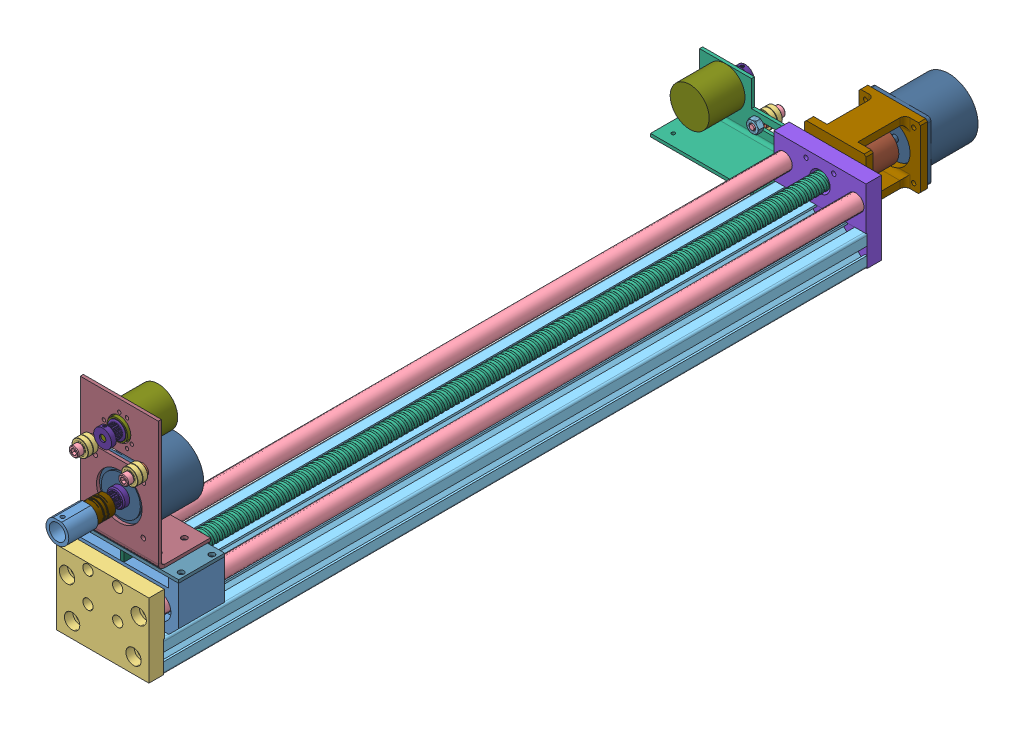
SolidWorks assembly BallScrewAssm2Motors, configuration Default. Lengths in mm.
Overall size (227 210 870.18).
53 component instances, 24 part files, 41 mates.
Components (placement in the parent):
- BallScrewBlock-1: BallScrewBlock [Default] at (0 32 293.5303) size (110 48 45)
- BallScrewCap-1: BallScrewCap [Default] at (0 51.5 283.5303) size (48.01 39 10)
- BallScrewEnd-1: BallScrewEnd [Default] at (0 36 357.5) x (-1 0 0) z (0 0 -1) size (90 72 15)
- BallScrewGuide-1: BallScrewGuide [Default] at (35 51.5 347.5) x (-0.923728 -0.383049 0) z (0.383049 -0.923728 0) size (16 705 16)
- Extrusion Base-1: Extrusion Base [Default] at origin size (90 30 687)
- BallScrewGuide-2: BallScrewGuide [Default] at (-35 51.5 347.5) x (-0.928239 -0.371985 0) z (0.371985 -0.928239 0) size (16 705 16)
- BallScrew-1: BallScrew [Default] at (0 51.5 347.5) x (-0.999726 0.023415 0) z (-0.023415 -0.999726 0) size (16.82 726.5 16)
- BallScrewBearing-1: BallScrewBearing [Default] at (0 51.5 342.5) x (1 0 0) z (0 -1 0) size (27 5 27)
- BallScrewMotorEnd-1: BallScrewMotorEnd [Default] at (0 36 -357.5) size (90 72 15)
- MotorMount-1: MotorMount [Default] at (0 51.5 -387.5) x (0 1 0) z (0 0 1) size (60 60 60)
- Motor-1: Motor [Default] at (0 51.5 -417.5) x (0 1 0) z (0 0 1) size (57.15 57.15 71.37)
- MotorBallCoupler-1: MotorBallCoupler [Default] at (0 51.5 -404.5) x (-0.999726 0.023415 0) z (0 0 1) size (30 30 34)
- CutPulley-1: CutPulley [Default] at (0 51.5 -404.5) x (0.023415 0.999726 0) z (-0.999726 0.023415 0) size (12.94 6.35 12.94)
- RodMotorAssm-1: RodMotorAssm [Default] at (0 86 316.0303) x (-1 0 0) z (0 0 -1) size (110 139 114.25)
  - HorizontalMotorMount-2: HorizontalMotorMount [Default] at origin size (76.2 127 50.8)
  - Motor-1: Motor [Default] at (0 41.45 -22.4) x (-1 0 0) z (0 0 -1) size (57.15 57.15 71.37)
  - MotorSupport-1: MotorSupport [Default] at (0 -6 0) size (110 3 45)
  - MotorPlatformSupport-1: MotorPlatformSupport [Default] at (0 -15 0) x (0 0 -1) z (1 0 0) size (45 12 3)
  - Encoder-1: Encoder [Default] at (0 98.6 12.6) x (-1 0 0) z (0 0 -1) size (38 38 53)
  - 1375K39_MXL Series Timing Belt Pulley-1: 1375K39_MXL Series Timing Belt Pulley [1375K39] at (0 41.45 -31.0741) x (0 0 -1) z (0.414927 -0.909855 0) size (14.3 17.4 17.4)
  - 6208K433_Clamping Precision Flexible Shaft Coupling-1: 6208K433_Clamping Precision Flexible Shaft Coupling [6208K433] at (0 41.45 -47.7492) size (20.03 19.05 19.05)
  - 1375K39_MXL Series Timing Belt Pulley-2: 1375K39_MXL Series Timing Belt Pulley [1375K39] at (0 98.6 -34.5501) x (0 0 1) z (0.089879 0.995953 0) size (14.3 17.4 17.4)
  - MotorRodCoupler-1: MotorRodCoupler [Default] at (0 41.45 -85.8492) x (-1 0 0) z (0 0 -1) size (22.23 21.43 38.1)
  - Idler-1: Idler [Default] at (25.4 75.7798 -30.4193) x (-0.670496 -0.741913 0) z (0 0 -1) size (15.88 15.88 29.4)
    - IdlerSpacer-1: IdlerSpacer [Default] at (0 0 -5.0193) x (1 0 0) z (0 -1 0) size (10.79 3 10.79)
    - 60355K701_Ball Bearing-1: 60355K701_Ball Bearing [60355K701] at (0 0 0.4699) size (15.88 15.88 4.98)
    - 91251A541_Black-Oxide Alloy Steel Socket Head Screw-1: 91251A541_Black-Oxide Alloy Steel Socket Head Screw [91251A541] at origin size (9.53 9.53 29.4)
    - 60355K701_Ball Bearing-2: 60355K701_Ball Bearing [60355K701] at (0 0 5.4483) size (15.88 15.88 4.98)
    - 95462A029_Medium-Strength Steel Hex Nut-1: 95462A029_Medium-Strength Steel Hex Nut [95462A029] at (0 0 -10.7974) size (11.11 12.83 6.51)
  - Idler-2: Idler [Default] at (-22.9813 75.7798 -30.4193) x (-0.670496 -0.741913 0) z (0 0 -1) size (15.88 15.88 29.4)
    - IdlerSpacer-1: IdlerSpacer [Default] at (0 0 -5.0193) x (1 0 0) z (0 -1 0) size (10.79 3 10.79)
    - 60355K701_Ball Bearing-1: 60355K701_Ball Bearing [60355K701] at (0 0 0.4699) size (15.88 15.88 4.98)
    - 91251A541_Black-Oxide Alloy Steel Socket Head Screw-1: 91251A541_Black-Oxide Alloy Steel Socket Head Screw [91251A541] at origin size (9.53 9.53 29.4)
    - 60355K701_Ball Bearing-2: 60355K701_Ball Bearing [60355K701] at (0 0 5.4483) size (15.88 15.88 4.98)
    - 95462A029_Medium-Strength Steel Hex Nut-1: 95462A029_Medium-Strength Steel Hex Nut [95462A029] at (0 0 -10.7974) size (11.11 12.83 6.51)
- BallEncoderAssm-1: BallEncoderAssm [Default] at (-45 3 -399.9402) x (-1 0 0) z (0 0 -1) size (131.66 50.8 70.38)
  - Encoder-1: Encoder [Default] at (101.6 28.75 -38) size (38 38 53)
  - BallEncoderHolder-1: BallEncoderHolder [Default] at origin size (127 50.8 50.8)
  - 1375K39_MXL Series Timing Belt Pulley-1: 1375K39_MXL Series Timing Belt Pulley [1375K39] at (101.6 28.75 9.1501) x (0 0 -1) z (1 0 0) size (14.3 17.4 17.4)
  - Idler-1: Idler [Default] at (6.35 12.875 5.0193) x (-0.556818 0.830635 0) z (0 0 1) size (15.88 15.88 29.4)
    - IdlerSpacer-1: IdlerSpacer [Default] at (0 0 -5.0193) x (1 0 0) z (0 -1 0) size (10.79 3 10.79)
    - 60355K701_Ball Bearing-1: 60355K701_Ball Bearing [60355K701] at (0 0 0.4699) size (15.88 15.88 4.98)
    - 91251A541_Black-Oxide Alloy Steel Socket Head Screw-1: 91251A541_Black-Oxide Alloy Steel Socket Head Screw [91251A541] at origin size (9.53 9.53 29.4)
    - 60355K701_Ball Bearing-2: 60355K701_Ball Bearing [60355K701] at (0 0 5.4483) size (15.88 15.88 4.98)
    - 95462A029_Medium-Strength Steel Hex Nut-1: 95462A029_Medium-Strength Steel Hex Nut [95462A029] at (0 0 -10.7974) size (11.11 12.83 6.51)
  - Idler-2: Idler [Default] at (69.85 12.875 5.0193) x (-0.099236 -0.995064 0) z (0 0 1) size (15.88 15.88 29.4)
    - IdlerSpacer-1: IdlerSpacer [Default] at (0 0 -5.0193) x (1 0 0) z (0 -1 0) size (10.79 3 10.79)
    - 60355K701_Ball Bearing-1: 60355K701_Ball Bearing [60355K701] at (0 0 0.4699) size (15.88 15.88 4.98)
    - 91251A541_Black-Oxide Alloy Steel Socket Head Screw-1: 91251A541_Black-Oxide Alloy Steel Socket Head Screw [91251A541] at origin size (9.53 9.53 29.4)
    - 60355K701_Ball Bearing-2: 60355K701_Ball Bearing [60355K701] at (0 0 5.4483) size (15.88 15.88 4.98)
    - 95462A029_Medium-Strength Steel Hex Nut-1: 95462A029_Medium-Strength Steel Hex Nut [95462A029] at (0 0 -10.7974) size (11.11 12.83 6.51)
  - 95462A029_Medium-Strength Steel Hex Nut-1: 95462A029_Medium-Strength Steel Hex Nut [95462A029] at (6.35 12.875 -5.7781) x (-0.99776 -0.066901 0) z (0 0 1) size (11.11 12.83 6.51)
  - 95462A029_Medium-Strength Steel Hex Nut-2: 95462A029_Medium-Strength Steel Hex Nut [95462A029] at (69.85 12.875 -5.7781) x (0.911368 0.411591 0) z (0 0 1) size (11.11 12.83 6.51)
Mates (geometry in assembly coordinates):
- Coincident1: coordinate: point of Extrusion Base-1
- Coincident2: coincident anti-aligned: plane of BallScrewEnd-1 through (0 36 343.5) normal (0 0 -1); plane of Extrusion Base-1 through (0 0 343.5) normal (0 0 1)
- Concentric1: concentric aligned: cylinder of BallScrewEnd-1 through (30 15 357.5) axis (0 0 1) radius 4.5; cylinder of Extrusion Base-1 through (30 15 343.5) axis (0 0 1) radius 3.5
- Concentric2: concentric aligned: cylinder of BallScrewEnd-1 through (-30 15 357.5) axis (0 0 1) radius 4.5; cylinder of Extrusion Base-1 through (-30 15 343.5) axis (0 0 1) radius 3.5
- Concentric3: concentric aligned: cylinder of BallScrewEnd-1 through (35 51.5 357.5) axis (0 0 1) radius 4.5; cylinder of BallScrewGuide-1 through (35 51.5 347.5) axis (0 0 1) radius 3.5
- Coincident3: coincident aligned: plane of BallScrewEnd-1 through (35 51.5 347.5) normal (0 0 -1); circle of BallScrewGuide-1
- Concentric4: concentric aligned: cylinder of BallScrewBlock-1 through (35 51.5 293.5303) axis (0 0 1) radius 8; cylinder of BallScrewGuide-1 through (35 51.5 -357.5) axis (0 0 1) radius 8
- Concentric5: concentric anti-aligned: cylinder of BallScrewBlock-1 through (0 51.5 293.5303) axis (0 0 1) radius 8; cylinder of BallScrewCap-1 through (0 51.5 293.5303) axis (0 0 -1) radius 8
- Coincident4: coincident: plane of BallScrewBlock-1 through (0 32 293.5303) normal (0 0 -1); line of BallScrewCap-1 through (14 71 293.5303) axis (-1 0 0)
- Concentric6: concentric anti-aligned: cylinder of BallScrewBlock-1 through (-13.435 64.935 293.5303) axis (0 0 -1) radius 2.5; cylinder of BallScrewCap-1 through (-13.435 64.935 293.5303) axis (0 0 1) radius 3.3
- Concentric7: concentric anti-aligned: cylinder of BallScrewEnd-1 through (-35 51.5 347.5) axis (0 0 -1) radius 8; cylinder of BallScrewGuide-2 through (-35 51.5 -357.5) axis (0 0 1) radius 8
- Coincident5: coincident aligned: plane of BallScrewEnd-1 through (-35 51.5 347.5) normal (0 0 -1); circle of BallScrewGuide-2
- Concentric8: concentric aligned: cylinder of BallScrewBlock-1 through (-35 51.5 293.5303) axis (0 0 1) radius 8; cylinder of BallScrewGuide-2 through (-35 51.5 -357.5) axis (0 0 1) radius 8
- Concentric9: concentric anti-aligned: cylinder of BallScrewEnd-1 through (0 51.5 347.5) axis (0 0 -1) radius 13.5; cylinder of BallScrew-1 through (0 51.5 342.5) axis (0 0 1) radius 7.25
- Coincident6: coincident anti-aligned: plane of BallScrewEnd-1 through (0 51.5 347.5) normal (0 0 -1); plane of BallScrew-1 through (0 51.5 347.5) normal (0 0 1)
- Concentric10: concentric anti-aligned: cylinder of BallScrew-1 through (0 51.5 342.5) axis (0 0 1) radius 7.25; cylinder of BallScrewBearing-1 through (0 51.5 347.5) axis (0 0 -1) radius 7.5
- Coincident7: coincident anti-aligned: plane of BallScrewEnd-1 through (0 51.5 347.5) normal (0 0 -1); circle of BallScrewBearing-1
- Concentric11: concentric aligned: cylinder of BallScrewGuide-1 through (35 51.5 -357.5) axis (0 0 1) radius 8; cylinder of BallScrewMotorEnd-1 through (35 51.5 -357.5) axis (0 0 1) radius 8
- Concentric12: concentric aligned: cylinder of BallScrewGuide-2 through (-35 51.5 -357.5) axis (0 0 1) radius 8; cylinder of BallScrewMotorEnd-1 through (-35 51.5 -357.5) axis (0 0 1) radius 8
- Coincident8: coincident anti-aligned: plane of Extrusion Base-1 through (0 0 -343.5) normal (0 0 -1); plane of BallScrewMotorEnd-1 through (0 36 -343.5) normal (0 0 1)
- Concentric13: concentric anti-aligned: cylinder of MotorMount-1 through (-13.5 38 -357.5) axis (0 0 1) radius 2.75; cylinder of BallScrewMotorEnd-1 through (-13.5 38 -357.5) axis (0 0 -1) radius 2.1
- Concentric14: concentric anti-aligned: cylinder of MotorMount-1 through (-13.5 65 -357.5) axis (0 0 1) radius 2.75; cylinder of BallScrewMotorEnd-1 through (-13.5 65 -357.5) axis (0 0 -1) radius 2.1
- Coincident9: coincident anti-aligned: plane of BallScrewMotorEnd-1 through (0 36 -357.5) normal (0 0 -1); plane of MotorMount-1 through (30 81.5 -357.5) normal (0 0 1)
- Concentric15: concentric aligned: cylinder of MotorMount-1 through (0 51.5 -417.5) axis (0 0 1) radius 20; cylinder of Motor-1 through (0 51.5 -468.3) axis (0 0 1) radius 28.575
- Concentric16: concentric anti-aligned: circle of MotorMount-1; circle of Motor-1
- Coincident10: coincident: plane of MotorMount-1 through (30 81.5 -417.5) normal (0 0 -1); line of Motor-1 through (-28.575 76.9 -417.5) axis (0 -1 0)
- Concentric17: concentric anti-aligned: cylinder of Motor-1 through (0 51.5 -396.926) axis (0 0 -1) radius 3.175; cylinder of MotorBallCoupler-1 through (0 51.5 -370.5) axis (0 0 1) radius 3.175
- Distance1: distance = 6 mm anti-aligned: plane of MotorMount-1 through (-30 81.5 -364.5) normal (0 0 -1); plane of MotorBallCoupler-1 through (0 51.5 -370.5) normal (0 0 1)
- Screw1: screw = 10 mm anti-aligned: cylinder of BallScrewBlock-1 through (0 51.5 328.5303) axis (0 0 1) radius 14.5; cylinder of BallScrew-1 through (0 51.5 -345) axis (0 0 -1) radius 7.25
- Concentric18: concentric anti-aligned: cylinder of Motor-1 through (0 51.5 -396.926) axis (0 0 -1) radius 3.175; cylinder of CutPulley-1 through (0 51.5 -410.85) axis (0 0 1) radius 3.175
- Coincident11: coincident aligned: plane of MotorBallCoupler-1 through (0 51.5 -404.5) normal (0 0 -1); circle of CutPulley-1
- Coincident12: coincident aligned: plane of BallScrew-1 through (0 51.5 347.5) normal (-0.023415 -0.999726 0); plane of MotorBallCoupler-1 through (0 51.5 -404.5) normal (-0.023415 -0.999726 0)
- Coincident13: coincident aligned: plane of MotorBallCoupler-1 through (0 51.5 -404.5) normal (-0.999726 0.023415 0); plane of CutPulley-1 through (0 51.5 -404.5) normal (-0.999726 0.023415 0)
- Concentric19: concentric aligned: cylinder of BallScrewBlock-1 through (-50 80 331.0303) axis (0 1 0) radius 2.5; cylinder of RodMotorAssm-1/MotorSupport-1 through (-50 83 331.0303) axis (0 1 0) radius 2.75
- Concentric20: concentric aligned: cylinder of BallScrewBlock-1 through (50 80 301.0303) axis (0 1 0) radius 2.5; cylinder of RodMotorAssm-1/MotorSupport-1 through (50 83 301.0303) axis (0 1 0) radius 2.75
- Coincident14: coincident anti-aligned: plane of BallScrewBlock-1 through (-55 80 338.5303) normal (0 1 0); plane of RodMotorAssm-1/MotorSupport-1 through (0 80 316.0303) normal (0 -1 0)
- Coincident15: coincident aligned: plane of BallScrewMotorEnd-1 through (-45 0 -342.5) normal (0 -1 0); plane of BallEncoderAssm-1/BallEncoderHolder-1 through (-45 0 -399.9402) normal (0 -1 0)
- Coincident16: coincident aligned: plane of MotorMount-1 through (-30 81.5 -410.5) normal (0 0 1); plane of BallEncoderAssm-1/1375K39_MXL Series Timing Belt Pulley-1 through (-146.6 24.1427 -410.5) normal (0 0 1)
- Coincident17: coincident anti-aligned: plane of BallScrewMotorEnd-1 through (-45 0 -342.5) normal (-1 0 0); plane of BallEncoderAssm-1/BallEncoderHolder-1 through (-45 0 -399.9402) normal (1 0 0)
- Coincident19: coincident anti-aligned: plane of RodMotorAssm-1/HorizontalMotorMount-2 through (0 86 338.4303) normal (0 0 -1); plane of 95462A029_Medium-Strength Steel Hex Nut-1 through (-21.7189 161.7798 338.4303) normal (0 0 1)
- Parallel1: parallel anti-aligned: plane of RodMotorAssm-1/Motor-1 through (-28.575 156.025 333.6043) normal (0 1 0); plane of 95462A029_Medium-Strength Steel Hex Nut-1 through (-18.511 156.2236 338.4303) normal (0 -1 0)
